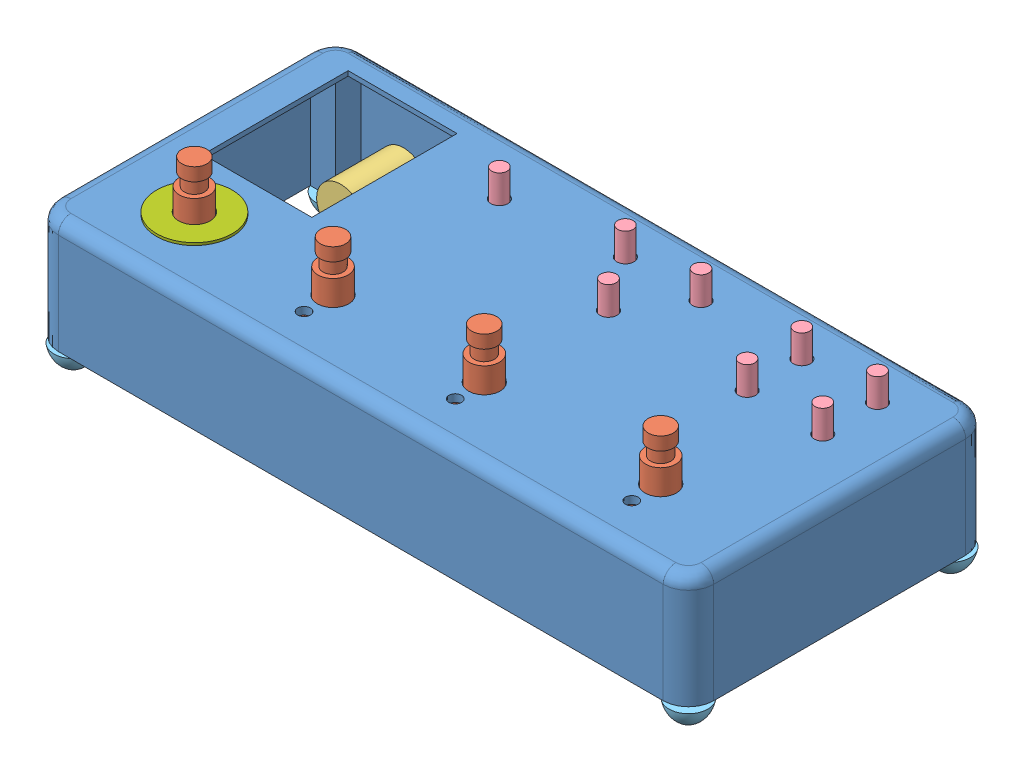
SolidWorks assembly 装配体221, configuration 默认. Lengths in mm.
Overall size (265.3 75 126.65).
22 component instances, 8 part files, 54 mates.
Components (placement in the parent):
- 上盖-1: 上盖 [默认] at (-65.3929 -23.5714 -20.5085) size (260 45 120)
- 踩钉-1: 踩钉 [默认] at (23.6371 3.8286 35.8963) x (0.016192 0 0.999869) z (-0.999869 0 0.016192) size (18 42.1 19.6)
- 踩钉-2: 踩钉 [默认] at (-46.3629 3.8286 35.8963) size (18 42.1 19.6)
- 踩钉-3: 踩钉 [默认] at (-106.3629 3.8286 35.8963) size (18 42.1 19.6)
- 踩钉-4: 踩钉 [默认] at (-161.3629 3.8286 35.8963) x (0 0 -1) z (1 0 0) size (18 42.1 19.6)
- 音频口-1: 音频口 [默认] at (-166.3629 -11.5714 -52.1037) x (-0.890749 0.454496 0) z (-0.454496 -0.890749 0) size (19 32 19)
- 音频口-2: 音频口 [默认] at (30.6371 -11.5714 -52.1037) x (1 0 0) z (0 1 0) size (19 32 19)
- 旋钮-1: 旋钮 [默认] at (-106.3629 4.3395 -36.325) x (0 -1 0) z (-1 0 0) size (28.5 11.1 11)
- 旋钮-2: 旋钮 [默认] at (-61.3629 4.3395 -41.325) x (0 -1 0) z (-1 0 0) size (28.5 11.1 11)
- 旋钮-3: 旋钮 [默认] at (-46.3629 4.3395 -19.5958) x (0 -1 0) z (-1 0 0) size (28.5 11.1 11)
- 旋钮-4: 旋钮 [默认] at (38.6371 4.3395 -41.325) x (0 -1 0) z (-1 0 0) size (28.5 11.1 11)
- 旋钮-5: 旋钮 [默认] at (-31.3629 4.3395 -41.325) x (0 -1 0) z (-1 0 0) size (28.5 11.1 11)
- 旋钮-6: 旋钮 [默认] at (38.6371 4.3395 -19.5958) x (0 -1 0) z (-1 0 0) size (28.5 11.1 11)
- 旋钮-7: 旋钮 [默认] at (8.6371 4.3395 -19.5958) x (0 -1 0) z (-1 0 0) size (28.5 11.1 11)
- 旋钮-8: 旋钮 [默认] at (8.6371 4.3395 -41.325) x (0 -1 0) z (-1 0 0) size (28.5 11.1 11)
- 底盖-1: 底盖 [默认] at (-66.3629 -25.5714 4.8963) size (260 2 120) (hidden)
- 脚垫-1: 脚垫 [默认] at (-184.0242 -21.7676 -47.1037) x (1 0 0) z (0 -1 0) size (15.39 15.39 23)
- 脚垫-2: 脚垫 [默认] at (-191.9952 -21.7676 54.5232) x (-0.837169 0 -0.546944) z (0 -1 0) size (15.39 15.39 23)
- 脚垫-3: 脚垫 [默认] at (52.0048 -21.7676 -49.4768) x (-0.837169 0 -0.546944) z (0 -1 0) size (15.39 15.39 23)
- 脚垫-4: 脚垫 [默认] at (52.0048 -21.7676 54.5232) x (-0.837169 0 -0.546944) z (0 -1 0) size (15.39 15.39 23)
- 3D_PCB1_2023-12-26new-1: 3D_PCB1_2023-12-26new [默认] at (-130.4322 -19.1714 34.3752) x (1 0 0) z (0 1 0) size (139.17 89.35 15)
- 散光片-1: 散光片 [默认] at (-161.3629 21.4286 35.8963) size (30 1 30)
Mates (geometry in assembly coordinates):
- 重合6: coincident anti-aligned: plane of 上盖-1 through (-65.3929 18.4286 -20.5085) normal (0 -1 0); plane of 踩钉-1 through (23.6371 18.4286 35.8963) normal (0 1 0)
- 同心2: concentric aligned: cylinder of 上盖-1 through (23.6371 21.4286 35.8963) axis (0 -1 0) radius 6.25; cylinder of 踩钉-1 through (23.6371 31.2286 35.8963) axis (0 -1 0) radius 6
- 重合7: coincident anti-aligned: plane of 上盖-1 through (-65.3929 18.4286 -20.5085) normal (0 -1 0); plane of 踩钉-2 through (-46.3629 18.4286 35.8963) normal (0 1 0)
- 同心3: concentric anti-aligned: circle of 上盖-1; cylinder of 踩钉-2 through (-46.3629 31.2286 35.8963) axis (0 -1 0) radius 6
- 重合8: coincident anti-aligned: plane of 上盖-1 through (-65.3929 18.4286 -20.5085) normal (0 -1 0); plane of 踩钉-3 through (-106.3629 18.4286 35.8963) normal (0 1 0)
- 同心4: concentric aligned: cylinder of 上盖-1 through (-106.3629 21.4286 35.8963) axis (0 -1 0) radius 6.25; cylinder of 踩钉-3 through (-106.3629 31.2286 35.8963) axis (0 -1 0) radius 6
- 重合9: coincident anti-aligned: plane of 上盖-1 through (-65.3929 18.4286 -20.5085) normal (0 -1 0); plane of 踩钉-4 through (-161.3629 18.4286 35.8963) normal (0 1 0)
- 同心5: concentric aligned: cylinder of 上盖-1 through (-161.3629 21.4286 35.8963) axis (0 -1 0) radius 6.25; cylinder of 踩钉-4 through (-161.3629 31.2286 35.8963) axis (0 -1 0) radius 6
- 平行2: parallel: plane of 上盖-1 through (60.6371 299.8384 61.8963) normal (0 0 -1); line of 踩钉-3 through (-114.9629 3.8286 45.6963) axis (1 0 0)
- 平行3: parallel aligned: plane of 上盖-1 through (-196.3629 21.4286 64.8963) normal (0 0 1); plane of 踩钉-4 through (-171.1629 18.4286 44.4963) normal (0 0 1)
- 同心6: concentric aligned: cylinder of 上盖-1 through (-166.3629 -11.5714 -58.1037) axis (0 0 1) radius 5; cylinder of 音频口-1 through (-166.3629 -11.5714 -59.1037) axis (0 0 1) radius 4.75
- 重合13: coincident anti-aligned: plane of 上盖-1 through (60.6371 299.8384 -52.1037) normal (0 0 1); plane of 音频口-1 through (-166.3629 -11.5714 -52.1037) normal (0 0 -1)
- 同心7: concentric anti-aligned: cylinder of 上盖-1 through (30.6371 -11.5714 -58.1037) axis (0 0 1) radius 5; cylinder of 音频口-2 through (30.6371 -11.5714 -27.1037) axis (0 0 -1) radius 9.5
- 重合14: coincident anti-aligned: plane of 上盖-1 through (60.6371 299.8384 -52.1037) normal (0 0 1); plane of 音频口-2 through (30.6371 -11.5714 -52.1037) normal (0 0 -1)
- 同心8: concentric aligned: cylinder of 上盖-1 through (-106.3629 21.4286 -30.1037) axis (0 -1 0) radius 3.4; cylinder of 旋钮-1 through (-106.3629 32.4286 -30.1037) axis (0 -1 0) radius 3.05
- 平行4: parallel: line of 上盖-1 through (-101.7629 18.4286 -36.1037) axis (0 0 1); plane of 旋钮-1 through (-101.5645 19.4286 -25.225) normal (1 0 0)
- 重合16: coincident anti-aligned: plane of 上盖-1 through (-65.3929 19.4286 -20.5085) normal (0 -1 0); plane of 旋钮-1 through (-101.5645 19.4286 -25.225) normal (0 1 0)
- 同心9: concentric aligned: circle of 上盖-1; cylinder of 旋钮-8 through (8.6371 32.4286 -35.1037) axis (0 -1 0) radius 3.05
- 同心10: concentric anti-aligned: circle of 上盖-1; cylinder of 旋钮-7 through (8.6371 32.4286 -13.3745) axis (0 -1 0) radius 3.05
- 同心11: concentric anti-aligned: circle of 上盖-1; cylinder of 旋钮-6 through (38.6371 32.4286 -13.3745) axis (0 -1 0) radius 3.05
- 同心12: concentric anti-aligned: circle of 上盖-1; cylinder of 旋钮-4 through (38.6371 32.4286 -35.1037) axis (0 -1 0) radius 3.05
- 同心13: concentric aligned: cylinder of 上盖-1 through (-31.3629 21.4286 -35.1037) axis (0 -1 0) radius 3.4; cylinder of 旋钮-5 through (-31.3629 32.4286 -35.1037) axis (0 -1 0) radius 3.05
- 同心14: concentric aligned: circle of 上盖-1; cylinder of 旋钮-2 through (-61.3629 32.4286 -35.1037) axis (0 -1 0) radius 3.05
- 同心15: concentric aligned: cylinder of 上盖-1 through (-46.3629 21.4286 -13.3745) axis (0 -1 0) radius 3.4; cylinder of 旋钮-3 through (-46.3629 32.4286 -13.3745) axis (0 -1 0) radius 3.05
- 平行5: parallel: line of 上盖-1 through (-50.9629 18.4286 -19.3745) axis (1 0 0); plane of 旋钮-3 through (-46.3629 4.3395 -19.5958) normal (0 0 -1)
- 平行6: parallel anti-aligned: plane of 上盖-1 through (-56.7629 19.4286 -41.1037) normal (0 0 1); plane of 旋钮-2 through (-61.3629 4.3395 -41.325) normal (0 0 -1)
- 平行7: parallel: line of 上盖-1 through (-35.9629 18.4286 -41.1037) axis (1 0 0); plane of 旋钮-5 through (-31.3629 4.3395 -41.325) normal (0 0 -1)
- 平行8: parallel: line of 上盖-1 through (4.0371 18.4286 -41.1037) axis (1 0 0); plane of 旋钮-8 through (8.6371 4.3395 -41.325) normal (0 0 -1)
- 平行9: parallel anti-aligned: plane of 上盖-1 through (13.2371 19.4286 -19.3745) normal (0 0 1); plane of 旋钮-7 through (8.6371 4.3395 -19.5958) normal (0 0 -1)
- 平行10: parallel anti-aligned: plane of 上盖-1 through (43.2371 19.4286 -19.3745) normal (0 0 1); plane of 旋钮-6 through (38.6371 4.3395 -19.5958) normal (0 0 -1)
- 平行11: parallel anti-aligned: plane of 上盖-1 through (43.2371 19.4286 -41.1037) normal (0 0 1); plane of 旋钮-4 through (38.6371 4.3395 -41.325) normal (0 0 -1)
- 重合24: coincident anti-aligned: plane of 上盖-1 through (-65.3929 19.4286 -20.5085) normal (0 -1 0); plane of 旋钮-2 through (-56.5645 19.4286 -30.225) normal (0 1 0)
- 重合25: coincident anti-aligned: plane of 上盖-1 through (-65.3929 19.4286 -20.5085) normal (0 -1 0); plane of 旋钮-5 through (-26.5645 19.4286 -30.225) normal (0 1 0)
- 重合26: coincident anti-aligned: plane of 上盖-1 through (-65.3929 19.4286 -20.5085) normal (0 -1 0); plane of 旋钮-3 through (-41.5645 19.4286 -8.4958) normal (0 1 0)
- 重合27: coincident anti-aligned: plane of 上盖-1 through (-65.3929 19.4286 -20.5085) normal (0 -1 0); plane of 旋钮-7 through (13.4355 19.4286 -8.4958) normal (0 1 0)
- 重合28: coincident anti-aligned: plane of 上盖-1 through (-65.3929 19.4286 -20.5085) normal (0 -1 0); plane of 旋钮-6 through (43.4355 19.4286 -8.4958) normal (0 1 0)
- 重合29: coincident anti-aligned: plane of 上盖-1 through (-65.3929 19.4286 -20.5085) normal (0 -1 0); plane of 旋钮-8 through (13.4355 19.4286 -30.225) normal (0 1 0)
- 重合30: coincident anti-aligned: plane of 上盖-1 through (-65.3929 19.4286 -20.5085) normal (0 -1 0); plane of 旋钮-4 through (43.4355 19.4286 -30.225) normal (0 1 0)
- 同心16: concentric anti-aligned: cylinder of 上盖-1 through (-188.3629 27.621 -47.1037) axis (0 -1 0) radius 3.25; circle of 底盖-1
- 同心17: concentric anti-aligned: cylinder of 上盖-1 through (-188.3629 27.621 56.8963) axis (0 -1 0) radius 3.25; cylinder of 底盖-1 through (-188.3629 -38.5714 56.8963) axis (0 1 0) radius 3.25
- 重合32: coincident anti-aligned: plane of 上盖-1 through (-65.3929 -23.5714 -20.5085) normal (0 -1 0); plane of 底盖-1 through (-186.3629 -23.5714 -45.1037) normal (0 1 0)
- 同心18: concentric anti-aligned: cylinder of 上盖-1 through (-188.3629 27.621 -47.1037) axis (0 -1 0) radius 3.25; cylinder of 脚垫-1 through (-188.3629 -5.4701 -47.1037) axis (0 1 0) radius 3.1962
- 重合33: coincident anti-aligned: plane of 底盖-1 through (-186.3629 -25.5714 -45.1037) normal (0 -1 0); plane of 脚垫-1 through (-184.0242 -25.5714 -47.1037) normal (0 1 0)
- 同心19: concentric aligned: cylinder of 底盖-1 through (-188.3629 -38.5714 56.8963) axis (0 1 0) radius 3.25; cylinder of 脚垫-2 through (-188.3629 -5.4701 56.8963) axis (0 1 0) radius 3.1962
- 重合34: coincident anti-aligned: plane of 底盖-1 through (-186.3629 -25.5714 -45.1037) normal (0 -1 0); plane of 脚垫-2 through (-191.9952 -25.5714 54.5232) normal (0 1 0)
- 同心20: concentric aligned: cylinder of 底盖-1 through (55.6371 -38.5714 56.8963) axis (0 1 0) radius 3.25; cylinder of 脚垫-4 through (55.6371 -5.4701 56.8963) axis (0 1 0) radius 3.1962
- 重合35: coincident anti-aligned: plane of 底盖-1 through (-186.3629 -25.5714 -45.1037) normal (0 -1 0); plane of 脚垫-4 through (52.0048 -25.5714 54.5232) normal (0 1 0)
- 同心21: concentric aligned: cylinder of 底盖-1 through (55.6371 -38.5714 -47.1037) axis (0 1 0) radius 3.25; cylinder of 脚垫-3 through (55.6371 -5.4701 -47.1037) axis (0 1 0) radius 3.1962
- 重合36: coincident anti-aligned: plane of 底盖-1 through (-186.3629 -25.5714 -45.1037) normal (0 -1 0); plane of 脚垫-3 through (52.0048 -25.5714 -49.4768) normal (0 1 0)
- 重合37: coincident anti-aligned: plane of 上盖-1 through (-65.3929 -17.5714 -20.5085) normal (0 -1 0); plane of 3D_PCB1_2023-12-26new-1 through (-60.8678 -17.5714 -8.5388) normal (0 1 0)
- 同心22: concentric aligned: cylinder of 上盖-1 through (-126.6222 -34.8851 -34.459) axis (0 1 0) radius 1.75; cylinder of 3D_PCB1_2023-12-26new-1 through (-126.6222 -19.1714 -34.459) axis (0 1 0) radius 1.75
- 同心23: concentric aligned: cylinder of 上盖-1 through (-127.1302 -34.8851 31.2002) axis (0 1 0) radius 1.75; cylinder of 3D_PCB1_2023-12-26new-1 through (-127.1302 -19.1714 31.2002) axis (0 1 0) radius 1.75
- 同心24: concentric aligned: cylinder of 踩钉-4 through (-161.3629 41.4286 35.8963) axis (0 -1 0) radius 5; cylinder of 散光片-1 through (-161.3629 22.4286 35.8963) axis (0 -1 0) radius 15
- 重合39: coincident anti-aligned: plane of 上盖-1 through (-65.3929 21.4286 -20.5085) normal (0 1 0); plane of 散光片-1 through (-161.3629 21.4286 35.8963) normal (0 -1 0)
